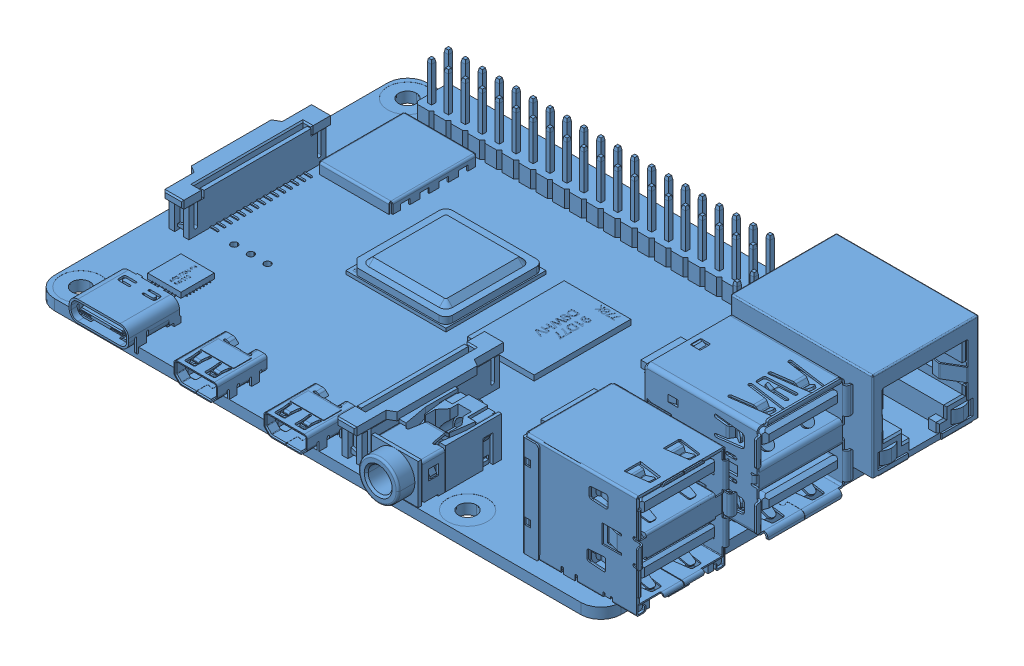
SolidWorks assembly raspberry pi 4, configuration Default. Lengths in mm.
Overall size (89 19.92 58.4).
2 component instances, 1 part files, 0 mates.
Components (placement in the parent):
- Assem_done(2)^2-1: Assem_done(2)^2 [Default] at origin size (89 19.92 58.4) (virtual)
  - Raspberry Pi 4 Model B^Assem_done(2)_2-1: Raspberry Pi 4 Model B^Assem_done(2)_2 [Default] at (50.9427 40.8 13.9283) size (89 19.92 58.4) (virtual)
